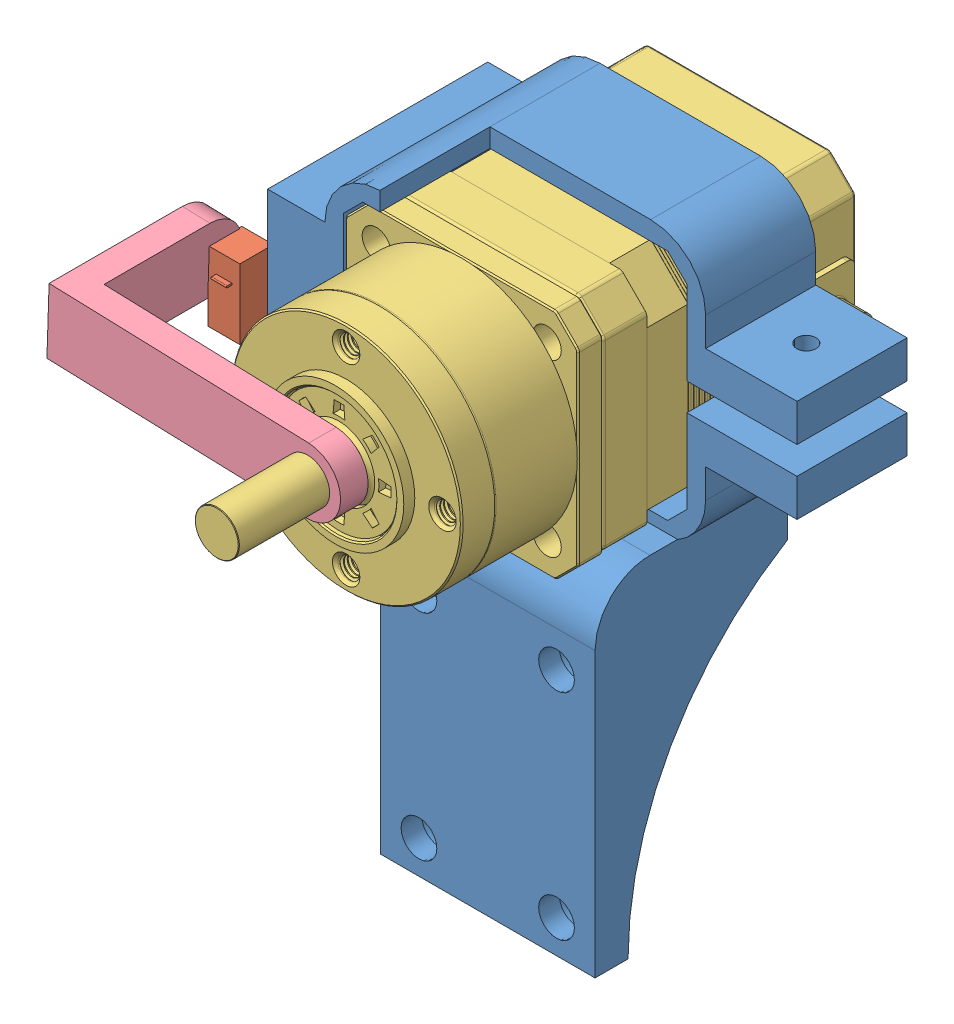
SolidWorks assembly Assem1, configuration Default. Lengths in mm.
Overall size (88.62 119.8 95.2).
4 component instances, 4 part files, 8 mates.
Components (placement in the parent):
- AOA-to-AL-block-stagger-endstop-collin-1: AOA-to-AL-block-stagger-endstop-collin [Mirror] at (-56.3363 46.0863 6.9872) size (86.2 119.8 40)
- endstop-1: endstop [Default] at (-91.3363 49.9863 35.4372) x (0 -1 0) z (-1 0 0) size (26.9 23.5 7.35)
- Correct_GearedStepper-1: Correct_GearedStepper [Default] at (-56.3863 46.1363 -13.8328) x (0 0 -1) z (1 0 0) size (95.2 42.3 53.3)
- GAP_AOA_LeverArm-1: GAP_AOA_LeverArm [Default] at (-56.3863 46.1363 64.6672) x (-0.032768 -0.999463 0) z (0 0 -1) size (12 53.2 30.23)
Mates (geometry in assembly coordinates):
- Coincident3: coincident anti-aligned: plane of AOA-to-AL-block-stagger-endstop-collin-1 through (-77.5363 24.8863 16.9872) normal (1 0 0); plane of Correct_GearedStepper-1 through (-77.5363 62.6863 32.1672) normal (-1 0 0)
- Coincident4: coincident anti-aligned: plane of AOA-to-AL-block-stagger-endstop-collin-1 through (-77.5363 67.2863 16.9872) normal (0 -1 0); plane of Correct_GearedStepper-1 through (-39.8363 67.2863 32.1672) normal (0 1 0)
- Distance1: distance = 10.82 mm aligned: plane of AOA-to-AL-block-stagger-endstop-collin-1 through (-56.3363 46.0863 -3.0128) normal (0 0 -1); plane of Correct_GearedStepper-1 through (-56.3863 46.1363 -13.8328) normal (0 0 -1)
- Concentric1: concentric anti-aligned: cylinder of Correct_GearedStepper-1 through (-56.3863 46.1363 81.1672) axis (0 0 -1) radius 4; cylinder of GAP_AOA_LeverArm-1 through (-56.3863 46.1363 59.6672) axis (0 0 1) radius 4
- Coincident6: coincident anti-aligned: plane of Correct_GearedStepper-1 through (-56.3863 46.1363 59.6672) normal (0 0 1); plane of GAP_AOA_LeverArm-1 through (-56.3863 46.1363 59.6672) normal (0 0 -1)
- Concentric2: concentric anti-aligned: cylinder of AOA-to-AL-block-stagger-endstop-collin-1 through (-91.3363 33.4863 31.9872) axis (1 0 0) radius 1.7; cylinder of endstop-1 through (-87.1863 33.4863 31.9872) axis (-1 0 0) radius 1.75
- Concentric5: concentric anti-aligned: cylinder of AOA-to-AL-block-stagger-endstop-collin-1 through (-91.3363 53.4863 31.9872) axis (1 0 0) radius 1.7; cylinder of endstop-1 through (-87.1863 53.4863 31.9872) axis (-1 0 0) radius 1.75
- Coincident7: coincident anti-aligned: plane of AOA-to-AL-block-stagger-endstop-collin-1 through (-91.3363 46.0863 6.9872) normal (-1 0 0); plane of endstop-1 through (-91.3363 53.4863 31.9872) normal (1 0 0)
